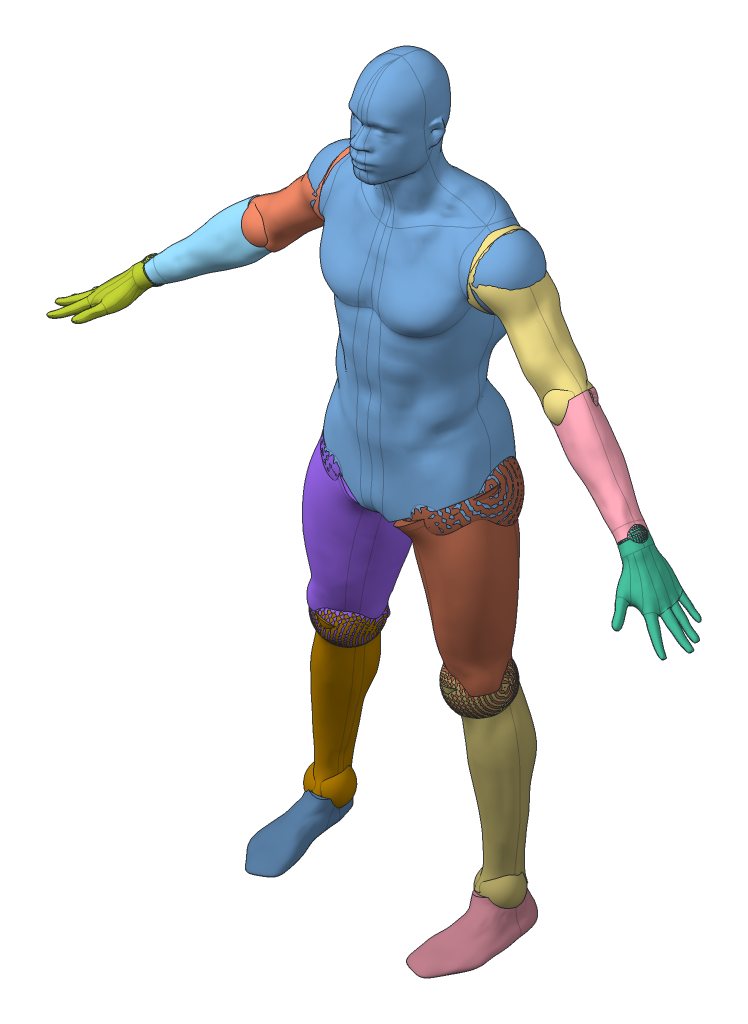
SolidWorks assembly Assem1, configuration Default. Lengths in mm.
Overall size (1585.65 1843.55 463.04).
13 component instances, 13 part files, 12 mates.
Components (placement in the parent):
- Body-no-hands-no-legs-1: Body-no-hands-no-legs [Default] at (-280.3466 -123.2784 796.9648) x (0.999982 0.004924 -0.003438) z (0.003454 -0.003201 0.999989) size (548.17 1062.75 308.36)
- levoe plecho12-1: levoe plecho12 [Default] at (-265.0997 -109.4623 810.1675) x (0.998587 0.047928 -0.022935) z (0.020533 0.050009 0.998538) size (349.64 316.91 182.66)
- levoe plecho1-1: levoe plecho1 [Default] at (-327.7463 -88.4083 802.6603) x (0.989807 -0.141482 0.016295) z (-0.012423 0.028202 0.999525) size (349.64 316.91 182.73)
- levoe predplecjie12-1: levoe predplecjie12 [Default] at (-312.6617 -122.7912 822.6818) x (0.995056 -0.068503 -0.071907) z (0.066667 -0.075924 0.994882) size (279.58 239.03 155.29)
- pravoe predplechie12-1: pravoe predplechie12 [Default] at (-267.1119 -105.5944 816.1908) x (0.998659 0.049898 -0.013775) z (0.010514 0.065045 0.997827) size (279.58 239.03 155.52)
- levaia kist1-1: levaia kist1 [Default] at (-304.4801 -111.45 887.2459) x (0.98133 -0.083235 -0.17339) z (0.154364 -0.196938 0.968188) size (215.98 173.92 183.55)
- pravaia kist 1-1: pravaia kist 1 [Default] at (-1411.7657 -119.1969 812.9909) x (0.999292 -0.028191 0.024897) z (-0.025513 -0.021703 0.999439) size (215.98 173.92 183.55)
- bedro2-1: bedro2 [Default] at (-280.9264 -125.0481 779.9825) x (-0.984969 0.021632 -0.171368) z (-0.166683 0.141137 0.975857) size (251.77 576.15 251.66)
- pravaia golen-1: pravaia golen [Default] at (-286.8002 -126.6286 710.4952) x (0.851228 -0.02336 -0.524275) z (0.524742 0.052131 0.849663) size (154.74 544.47 192.15)
- pravaia stopa-1: pravaia stopa [Default] at (-283.2827 -125.5323 747.866) x (0.76886 0.007134 -0.639377) z (0.639405 -0.002499 0.768866) size (190.69 129.27 280.13)
- bedro1-2: bedro1 [Default] at (-264.65 -120.5743 793.1319) x (0.930538 -0.015236 -0.365877) z (0.363873 0.150796 0.919161) size (251.77 576.15 251.66)
- levaia golen-1: levaia golen [Default] at (-283.2758 -132.8267 669.0919) x (0.799078 0.054658 0.598737) z (-0.601226 0.07056 0.795958) size (154.74 544.47 192.15)
- levaia stopa-1: levaia stopa [Default] at (-305.8309 -131.9873 785.8604) x (0.855739 0.020301 0.517009) z (-0.516919 -0.009873 0.855978) size (190.69 129.28 280.13)
Mates (geometry in assembly coordinates):
- Concentric7: concentric: sphere of Body-no-hands-no-legs-1; sphere of levoe plecho12-1
- Concentric8: concentric: sphere of Body-no-hands-no-legs-1; sphere of levoe plecho1-1
- Concentric9: concentric: sphere of levoe plecho12-1; sphere of pravoe predplechie12-1
- Concentric10: concentric: sphere of pravoe predplechie12-1; sphere of pravaia kist 1-1
- Concentric11: concentric: sphere of levoe plecho1-1; sphere of levoe predplecjie12-1
- Concentric12: concentric: sphere of levoe predplecjie12-1; sphere of levaia kist1-1
- Concentric16: concentric: sphere of Body-no-hands-no-legs-1; sphere of bedro2-1
- Concentric17: concentric: sphere of bedro2-1; sphere of pravaia golen-1
- Concentric18: concentric: sphere of pravaia golen-1; sphere of pravaia stopa-1
- Concentric19: concentric: sphere of Body-no-hands-no-legs-1; sphere of bedro1-2
- Concentric20: concentric: sphere of bedro1-2; sphere of levaia golen-1
- Concentric21: concentric: sphere of levaia golen-1; sphere of levaia stopa-1
